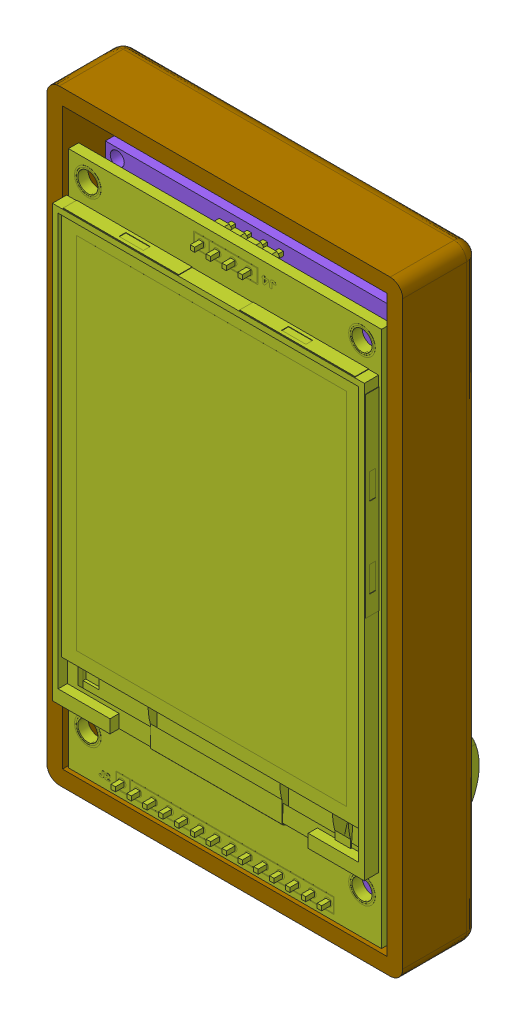
SolidWorks assembly BTCPOS.Solid_pcb, configuration Défaut. Lengths in mm.
Overall size (57 97 24.38).
37 component instances, 9 part files, 1 mates.
Components (placement in the parent):
- BTCPOS.Solid_pcb.step-1: BTCPOS.Solid_pcb.step [Défaut] at origin size (52.52 91.11 24.38)
  - C_0805_2012Metric.step-1: C_0805_2012Metric.step [Défaut] at (138.028 -96.52 -0.05) x (1 0 0) z (0 0 -1) size (2 1.25 1.25)
    - SOLID.step-1: SOLID.step [Défaut] at origin size (2 1.25 1.25)
  - C_0805_2012Metric.step-2: C_0805_2012Metric.step [Défaut] at (138.198 -104.14 -0.05) x (-1 0 0) z (0 0 -1) size (2 1.25 1.25)
    - SOLID.step-1: SOLID.step [Défaut] at origin size (2 1.25 1.25)
  - C_0805_2012Metric.step-3: C_0805_2012Metric.step [Défaut] at (150.092 -50.8 -0.05) x (1 0 0) z (0 0 -1) size (2 1.25 1.25)
    - SOLID.step-1: SOLID.step [Défaut] at origin size (2 1.25 1.25)
  - C_0805_2012Metric.step-4: C_0805_2012Metric.step [Défaut] at (152.4 -116.205 -0.05) x (1 0 0) z (0 0 -1) size (2 1.25 1.25)
    - SOLID.step-1: SOLID.step [Défaut] at origin size (2 1.25 1.25)
  - C_0805_2012Metric.step-5: C_0805_2012Metric.step [Défaut] at (152.4 -113.665 -0.05) x (-1 0 0) z (0 0 -1) size (2 1.25 1.25)
    - SOLID.step-1: SOLID.step [Défaut] at origin size (2 1.25 1.25)
  - USB Type C Port (SMD Type).step-1: USB Type C Port (SMD Type).step [Défaut] at (135.465 -113.665 -1.55) x (0 1 0) z (0 0 1) size (8.94 7.9 4.2)
    - COMPOUND.step-1: COMPOUND.step [Défaut] at origin size (8.94 7.9 4.2)
  - R_0805_2012Metric.step-1: R_0805_2012Metric.step [Défaut] at (143.51 -116.205 -0.05) x (-1 0 0) z (0 0 -1) size (2 1.2 0.45)
    - SOLID-0.step-1: SOLID-0.step [Défaut] at origin size (2 1.2 0.45)
  - R_0805_2012Metric.step-2: R_0805_2012Metric.step [Défaut] at (143.51 -113.665 -0.05) x (1 0 0) z (0 0 -1) size (2 1.2 0.45)
    - SOLID-0.step-1: SOLID-0.step [Défaut] at origin size (2 1.2 0.45)
  - R_0805_2012Metric.step-3: R_0805_2012Metric.step [Défaut] at (143.51 -118.745 -0.05) x (-1 0 0) z (0 0 -1) size (2 1.2 0.45)
    - SOLID-0.step-1: SOLID-0.step [Défaut] at origin size (2 1.2 0.45)
  - R_0805_2012Metric.step-4: R_0805_2012Metric.step [Défaut] at (143.51 -110.49 -0.05) x (-1 0 0) z (0 0 -1) size (2 1.2 0.45)
    - SOLID-0.step-1: SOLID-0.step [Défaut] at origin size (2 1.2 0.45)
  - R_0805_2012Metric.step-5: R_0805_2012Metric.step [Défaut] at (150.13 -45.72 -0.05) x (1 0 0) z (0 0 -1) size (2 1.2 0.45)
    - SOLID-0.step-1: SOLID-0.step [Défaut] at origin size (2 1.2 0.45)
  - SKRPABE010.step-1: SKRPABE010.step [Défaut] at (160.865 -75.5665 -0.05) x (1 0 0) z (0 1 0) size (4.6 2.5 3.2)
    - SOLID-1.step-1: SOLID-1.step [Défaut] at origin size (4.6 2.5 3.2)
  - SKRPABE010.step-2: SKRPABE010.step [Défaut] at (166.985 -75.5665 -0.05) x (1 0 0) z (0 1 0) size (4.6 2.5 3.2)
    - SOLID-1.step-1: SOLID-1.step [Défaut] at origin size (4.6 2.5 3.2)
  - SOT-223.step-1: SOT-223.step [Défaut] at (145.415 -100.33 -0.05) x (1 0 0) z (0 0 -1) size (7 6.5 1.7)
    - SOLID-2.step-1: SOLID-2.step [Défaut] at origin size (7 6.5 1.7)
  - ESP32-S2-WROVER.step-1: ESP32-S2-WROVER.step [Défaut] at (164.592 -52.324 -0.05) x (-1 0 0) z (0 0 -1) size (17.99 31 2.92)
    - COMPOUND-3.step-1: COMPOUND-3.step [Défaut] at origin size (17.99 31 2.92)
  - 2.8 TFT Module.step-1: 2.8 TFT Module.step [Défaut] at (153.88 -84.98 5.15) x (-1 0 0) z (0 0 1) size (51.88 85.9 24.38)
    - COMPOUND-4.step-1: COMPOUND-4.step [Défaut] at origin size (51.88 85.9 24.38)
  - R_0805_2012Metric.step-6: R_0805_2012Metric.step [Défaut] at (169.862 -117.602 -0.05) x (0 1 0) z (0 0 -1) size (2 1.2 0.45)
    - SOLID-0.step-1: SOLID-0.step [Défaut] at origin size (2 1.2 0.45)
  - COMPOUND-5.step-1: COMPOUND-5.step [Défaut] at origin size (48.26 83.82 1.6)
- coque inf-1: coque inf [Défaut] at (153.8518 -82.5742 -2.95) size (57 97 12.23)
Mates (geometry in assembly coordinates):
- Coïncidente1: coincident anti-aligned: plane of BTCPOS.Solid_pcb.step-1/ESP32-S2-WROVER.step-1/COMPOUND-3.step-1 through (164.592 -52.324 -2.95) normal (0 0 -1); plane of coque inf-1 through (153.8518 -82.5742 -2.95) normal (0 0 1)
